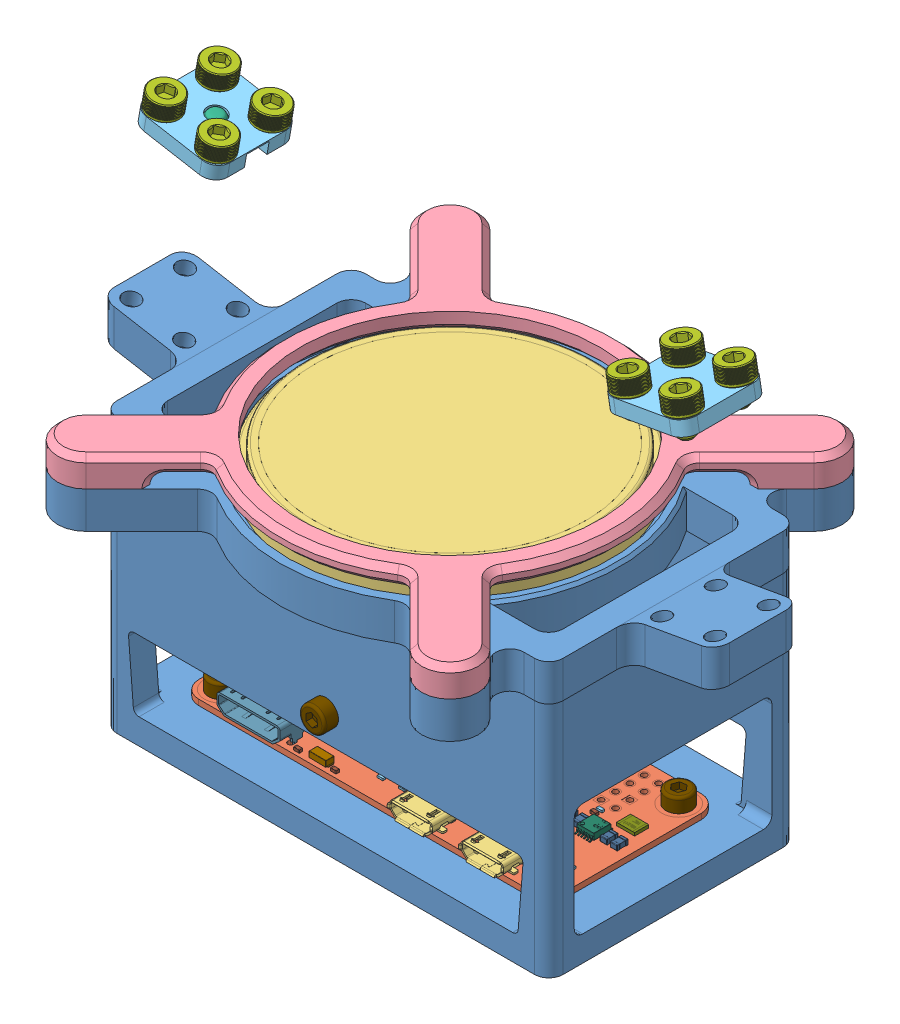
SolidWorks assembly Camera_Case_V1, configuration Default. Lengths in mm.
Overall size (109 86.17 76.19).
152 component instances, 36 part files, 45 mates.
Components (placement in the parent):
- FILTER_MOUNT-1: FILTER_MOUNT [Default] at (13.2312 42.9687 75.706) size (109 9.14 74.46)
- neodymium-1: neodymium [6x3] at (45.4614 49.3687 43.4758) x (0.944555 0 -0.328353) z (-0.328353 0 -0.944555) size (6 3 6)
- neodymium-10: neodymium [3x2] at (50.2312 42.9687 56.206) x (0.999996 0 0.002671) z (-0.002671 0 0.999996) size (3 2 3)
- LENS-1: LENS [Default] at (13.2312 47.4687 75.706) x (-0.754116 0 0.656742) z (-0.656742 0 -0.754116) size (54 5.6 54)
- FILTER_MOUNT_COVER-1: FILTER_MOUNT_COVER [Default] at (13.2312 49.4687 75.706) size (74.46 5 74.46)
- neodymium-2: neodymium [6x3] at (45.4614 49.4687 43.4758) x (-0.92324 0 -0.384223) z (0.384223 0 -0.92324) size (6 3 6)
- neodymium-3: neodymium [6x3] at (45.4614 49.3687 107.9363) x (0.944555 0 0.328353) z (0.328353 0 -0.944555) size (6 3 6)
- neodymium-4: neodymium [6x3] at (45.4614 49.4687 107.9363) x (-0.92324 0 0.384223) z (-0.384223 0 -0.92324) size (6 3 6)
- neodymium-5: neodymium [6x3] at (-18.9991 49.3687 43.4758) x (-0.944555 0 -0.328353) z (-0.328353 0 0.944555) size (6 3 6)
- neodymium-6: neodymium [6x3] at (-18.9991 49.3687 107.9363) x (-0.944555 0 0.328353) z (0.328353 0 0.944555) size (6 3 6)
- neodymium-7: neodymium [6x3] at (-18.9991 49.4687 107.9363) x (0.92324 0 0.384223) z (-0.384223 0 0.92324) size (6 3 6)
- neodymium-8: neodymium [6x3] at (-18.9991 49.4687 43.4758) x (0.92324 0 -0.384223) z (0.384223 0 0.92324) size (6 3 6)
- LED_COVER-1: LED_COVER [Default] at (54.5876 82.7974 75.706) x (0 0 -1) z (-0.984808 -0.173648 0) size (15 2.5 15)
- LED_COVER-2: LED_COVER [Default] at (-28.1253 82.7974 75.706) x (0 0 1) z (0.984808 -0.173648 0) size (15 2.5 15)
- SFH_4716AS_20151008_geometry-1: SFH_4716AS_20151008_geometry [Standard] at (-28.3361 81.6017 75.706) x (-0.984808 0.173648 0) z (0.173648 0.984808 0) size (3.75 3.75 1.55)
- SFH_4716AS_20151008_geometry-2: SFH_4716AS_20151008_geometry [Standard] at (54.7984 81.6017 75.706) x (-0.984808 -0.173648 0) z (-0.173648 0.984808 0) size (3.75 3.75 1.55)
- hex_socket_cylindrical_head_M3.0x4.step-1: hex_socket_cylindrical_head_M3.0x4.step [Default] at (-32.8899 83.1299 80.456) x (-0.968481 0.170769 -0.181335) z (0.173648 0.984808 0) size (5.5 5.5 7.01)
- hex_socket_cylindrical_head_M3.0x4.step-7: hex_socket_cylindrical_head_M3.0x4.step [Default] at (59.3523 83.1299 80.456) x (0.968481 0.170769 -0.181335) z (-0.173648 0.984808 0) size (5.5 5.5 7.01)
- hex_socket_cylindrical_head_M3.0x4.step-3: hex_socket_cylindrical_head_M3.0x4.step [Default] at (-23.5343 81.4802 80.456) x (0.968481 -0.170769 -0.181335) z (0.173648 0.984808 0) size (5.5 5.5 7.01)
- hex_socket_cylindrical_head_M3.0x4.step-8: hex_socket_cylindrical_head_M3.0x4.step [Default] at (49.9966 81.4802 80.456) x (-0.968481 -0.170769 -0.181335) z (-0.173648 0.984808 0) size (5.5 5.5 7.01)
- hex_socket_cylindrical_head_M3.0x4.step-2: hex_socket_cylindrical_head_M3.0x4.step [Default] at (-32.8899 83.1299 70.956) x (-0.968481 0.170769 0.181335) z (0.173648 0.984808 0) size (5.5 5.5 7.01)
- hex_socket_cylindrical_head_M3.0x4.step-6: hex_socket_cylindrical_head_M3.0x4.step [Default] at (59.3523 83.1299 70.956) x (0.968481 0.170769 0.181335) z (-0.173648 0.984808 0) size (5.5 5.5 7.01)
- hex_socket_cylindrical_head_M3.0x4.step-4: hex_socket_cylindrical_head_M3.0x4.step [Default] at (-23.5343 81.4802 70.956) x (0.968481 -0.170769 0.181335) z (0.173648 0.984808 0) size (5.5 5.5 7.01)
- hex_socket_cylindrical_head_M3.0x4.step-5: hex_socket_cylindrical_head_M3.0x4.step [Default] at (49.9966 81.4802 70.956) x (-0.968481 -0.170769 0.181335) z (-0.173648 0.984808 0) size (5.5 5.5 7.01)
- PI_CAM_MOUNT-1: PI_CAM_MOUNT [Default] at (13.2312 20.2317 75.706) x (-1 0 0) z (0 0 -1) size (24.75 5 38)
- M2x1.6mm Hex Nut.step-5: M2x1.6mm Hex Nut.step [Default] at (6.4812 20.3687 86.206) x (-0.866025 0 -0.5) z (0 1 0) size (4.63 4.63 1.6)
- M2x1.6mm Hex Nut.step-13: M2x1.6mm Hex Nut.step [Default] at (19.9812 21.9687 86.206) x (0.866025 0 -0.5) z (0 -1 0) size (4.63 4.63 1.6)
- M2x1.6mm Hex Nut.step-12: M2x1.6mm Hex Nut.step [Default] at (6.4812 21.9687 65.206) x (-0.866025 0 0.5) z (0 -1 0) size (4.63 4.63 1.6)
- M2x1.6mm Hex Nut.step-14: M2x1.6mm Hex Nut.step [Default] at (19.9812 20.3687 65.206) x (0.866025 0 0.5) z (0 1 0) size (4.63 4.63 1.6)
- M2x1.6mm Hex Nut.step-7: M2x1.6mm Hex Nut.step [Default] at (6.4812 21.9687 65.206) x (-0.866025 0 0.5) z (0 -1 0) size (4.63 4.63 1.6) (hidden)
- M2x1.6mm Hex Nut.step-6: M2x1.6mm Hex Nut.step [Default] at (19.9812 21.9687 86.206) x (0.866025 0 -0.5) z (0 -1 0) size (4.63 4.63 1.6) (hidden)
- M2x1.6mm Hex Nut.step-8: M2x1.6mm Hex Nut.step [Default] at (19.9812 20.3687 65.206) x (0.866025 0 0.5) z (0 1 0) size (4.63 4.63 1.6) (hidden)
- Camera Module Assem.STEP-1: Camera Module Assem.STEP [Default] at (-2.8699 5.7203 66.7324) x (0 0 1) z (0 1 0) size (25 24 24.98)
  - 15 Pin Ribbon Block Assem.STEP-1: 15 Pin Ribbon Block Assem.STEP [Default] at (0.7567 20.5462 10.9417) x (1 0 0) z (0 -1 0) size (22 2.5 7)
    - 15 Pin Ribbon Block.STEP-1: 15 Pin Ribbon Block.STEP [Default] at (8.217 10.8197 14.6952) size (20 2.5 6)
    - Ribbon Clamp.STEP-1: Ribbon Clamp.STEP [Default] at (8.217 10.8197 14.6952) size (22 2.5 5)
  - PCB 1.STEP-1: PCB 1.STEP [Default] at (8.9736 12.851 19.5114) size (25 24 2.1)
  - Camera Block.STEP-1: Camera Block.STEP [Default] at (8.9736 15.851 20.5114) size (22 13.5 12.5)
  - Camera end.STEP-1: Camera end.STEP [Default] at (8.9736 15.851 27.3922) x (0.999924 0.012337 0) z (0 0 1) size (14 14 17)
  - Lenz.STEP-1: Lenz.STEP [Default] at (8.9736 15.851 43.8922) size (9 9 0.5)
  - 0603 Resistor.STEP-1: 0603 Resistor.STEP [Default] at (2.3268 23.572 20.4882) size (1.75 0.85 0.59)
  - 0603 Resistor.STEP-2: 0603 Resistor.STEP [Default] at (4.5768 23.572 20.4882) size (1.75 0.85 0.59)
  - 0603 Resistor.STEP-3: 0603 Resistor.STEP [Default] at (15.6203 23.5707 20.4857) size (1.75 0.85 0.59)
  - 0603 Resistor.STEP-4: 0603 Resistor.STEP [Default] at (13.3703 23.5707 20.4857) size (1.75 0.85 0.59)
- hex_socket_cylindrical_head_M2.5x06.step-1: hex_socket_cylindrical_head_M2.5x06.step [Default] at (19.9812 26.3317 86.206) x (0.143858 0 0.989598) z (0 1 0) size (4.5 4.5 8.5)
- hex_socket_cylindrical_head_M2.5x06.step-3: hex_socket_cylindrical_head_M2.5x06.step [Default] at (6.4812 26.3317 86.206) x (-0.143858 0 0.989598) z (0 1 0) size (4.5 4.5 8.5)
- hex_socket_cylindrical_head_M2.5x06.step-2: hex_socket_cylindrical_head_M2.5x06.step [Default] at (19.9812 26.3317 65.206) x (0.143858 0 -0.989598) z (0 1 0) size (4.5 4.5 8.5)
- hex_socket_cylindrical_head_M2.5x06.step-4: hex_socket_cylindrical_head_M2.5x06.step [Default] at (6.4812 26.3317 65.206) x (-0.143858 0 -0.989598) z (0 1 0) size (4.5 4.5 8.5)
- hex_socket_cylindrical_head_M2.5x08.step-1: hex_socket_cylindrical_head_M2.5x08.step [Default] at (13.2312 22.7317 53.706) x (-0.82955 -0.558433 0) z (0 0 -1) size (4.5 4.5 10.5)
- neodymium-11: neodymium [3x2] at (50.2312 42.9687 95.206) x (0.999996 0 -0.002671) z (0.002671 0 0.999996) size (3 2 3)
- neodymium-13: neodymium [3x2] at (-23.7688 42.9687 56.206) x (-0.999996 0 0.002671) z (-0.002671 0 -0.999996) size (3 2 3)
- neodymium-15: neodymium [3x2] at (-23.7688 42.9687 95.206) x (-0.999996 0 -0.002671) z (0.002671 0 -0.999996) size (3 2 3)
- neodymium-9: neodymium [3x2] at (50.2312 40.9687 56.206) x (0.988314 0 0.152432) z (-0.152432 0 0.988314) size (3 2 3)
- neodymium-14: neodymium [3x2] at (-23.7688 40.9687 56.206) x (-0.988314 0 0.152432) z (-0.152432 0 -0.988314) size (3 2 3)
- neodymium-12: neodymium [3x2] at (50.2312 40.9687 95.206) x (0.988314 0 -0.152432) z (0.152432 0 0.988314) size (3 2 3)
- neodymium-16: neodymium [3x2] at (-23.7688 40.9687 95.206) x (-0.988314 0 -0.152432) z (0.152432 0 -0.988314) size (3 2 3)
- PI_CASE-1: PI_CASE [Default] at (13.2312 0.9687 75.706) size (79 42 44)
- M2x1.6mm Hex Nut.step-1: M2x1.6mm Hex Nut.step [Default] at (42.2312 2.9687 64.206) x (-0.866025 0 0.5) z (0 -1 0) size (4.63 4.63 1.6)
- M2x1.6mm Hex Nut.step-10: M2x1.6mm Hex Nut.step [Default] at (-15.7688 1.3687 64.206) x (0.866025 0 0.5) z (0 1 0) size (4.63 4.63 1.6)
- M2x1.6mm Hex Nut.step-9: M2x1.6mm Hex Nut.step [Default] at (42.2312 1.3687 87.206) x (-0.866025 0 -0.5) z (0 1 0) size (4.63 4.63 1.6)
- M2x1.6mm Hex Nut.step-11: M2x1.6mm Hex Nut.step [Default] at (-15.7688 2.9687 87.206) x (0.866025 0 -0.5) z (0 -1 0) size (4.63 4.63 1.6)
- M2x1.6mm Hex Nut.step-4: M2x1.6mm Hex Nut.step [Default] at (-15.7688 1.3687 64.206) x (0.866025 0 0.5) z (0 1 0) size (4.63 4.63 1.6) (hidden)
- M2x1.6mm Hex Nut.step-2: M2x1.6mm Hex Nut.step [Default] at (42.2312 1.3687 87.206) x (-0.866025 0 -0.5) z (0 1 0) size (4.63 4.63 1.6)
- M2x1.6mm Hex Nut.step-3: M2x1.6mm Hex Nut.step [Default] at (-15.7688 2.9687 87.206) x (0.866025 0 -0.5) z (0 -1 0) size (4.63 4.63 1.6) (hidden)
- RPi Zero.stp-1: RPi Zero.stp [Default] at (64.4875 -14.6279 62.6518) size (67.53 4.45 31.23)
  - Raspberry_pizero_PCB.stp-1: Raspberry_pizero_PCB.stp [Default] at (-51.2564 20.0966 13.0542) size (65 1 30)
  - Micro USB_input_female (short)-SMT.stp-1: Micro USB_input_female (short)-SMT.stp [Default] at (-42.3564 22.3216 26.5042) size (7.98 2.94 5.43)
  - Micro USB_input_female (short)-SMT.stp-2: Micro USB_input_female (short)-SMT.stp [Default] at (-29.7564 22.3216 26.5042) size (7.98 2.94 5.43)
  - 0204 - Capacitor.stp-1: 0204 - Capacitor.stp [Default] at (-62.4121 21.3466 11.2398) size (1 0.5 0.6)
  - 0204 - Capacitor.stp-2: 0204 - Capacitor.stp [Default] at (-62.4121 21.3466 12.2528) size (1 0.5 0.6)
  - 0204 - Capacitor.stp-3: 0204 - Capacitor.stp [Default] at (-61.8122 21.3466 13.3136) size (1 0.5 0.6)
  - 0204 - Capacitor.stp-4: 0204 - Capacitor.stp [Default] at (-61.8122 21.3466 14.2646) size (1 0.5 0.6)
  - 0204 - Capacitor.stp-5: 0204 - Capacitor.stp [Default] at (-61.8122 21.3466 15.241) size (1 0.5 0.6)
  - 0204 - Capacitor.stp-6: 0204 - Capacitor.stp [Default] at (-61.8122 21.3466 16.2144) size (1 0.5 0.6)
  - 0204 - Capacitor.stp-7: 0204 - Capacitor.stp [Default] at (-61.8122 21.3466 17.2416) size (1 0.5 0.6)
  - 0204 - Capacitor.stp-8: 0204 - Capacitor.stp [Default] at (-62.5919 21.3466 20.9695) size (1 0.5 0.6)
  - 0204 - Capacitor.stp-9: 0204 - Capacitor.stp [Default] at (-62.5919 21.3466 21.919) size (1 0.5 0.6)
  - 0204 - Capacitor.stp-10: 0204 - Capacitor.stp [Default] at (-60.4584 21.3466 22.3712) x (0 0 1) z (-1 0 0) size (1 0.5 0.6)
  - 0204 - Capacitor.stp-11: 0204 - Capacitor.stp [Default] at (-60.0807 21.3466 22.3712) x (0 0 -1) z (1 0 0) size (1 0.5 0.6)
  - 0204 - Capacitor.stp-12: 0204 - Capacitor.stp [Default] at (-59.0466 21.3466 22.3712) x (0 0 -1) z (1 0 0) size (1 0.5 0.6)
  - 0204 - Capacitor.stp-13: 0204 - Capacitor.stp [Default] at (-52.6496 21.3466 22.316) x (0 0 1) z (-1 0 0) size (1 0.5 0.6)
  - 0204 - Capacitor.stp-14: 0204 - Capacitor.stp [Default] at (-52.25 21.3466 22.316) x (0 0 -1) z (1 0 0) size (1 0.5 0.6)
  - 0204 - Capacitor.stp-15: 0204 - Capacitor.stp [Default] at (-51.2398 21.3466 22.316) x (0 0 -1) z (1 0 0) size (1 0.5 0.6)
  - 0204 - Capacitor.stp-16: 0204 - Capacitor.stp [Default] at (-49.1841 21.3466 22.316) x (0 0 -1) z (1 0 0) size (1 0.5 0.6)
  - 0204 - Capacitor.stp-17: 0204 - Capacitor.stp [Default] at (-48.1448 21.3466 22.316) x (0 0 -1) z (1 0 0) size (1 0.5 0.6)
  - 0204 - Capacitor.stp-18: 0204 - Capacitor.stp [Default] at (-46.475 21.3466 21.113) size (1 0.5 0.6)
  - 0204 - Capacitor.stp-19: 0204 - Capacitor.stp [Default] at (-45.7322 21.3466 20.0663) size (1 0.5 0.6)
  - 0204 - Capacitor.stp-20: 0204 - Capacitor.stp [Default] at (-45.7322 21.3466 19.0675) size (1 0.5 0.6)
  - 0204 - Capacitor.stp-21: 0204 - Capacitor.stp [Default] at (-45.7322 21.3466 18.1249) size (1 0.5 0.6)
  - 0204 - Capacitor.stp-22: 0204 - Capacitor.stp [Default] at (-45.7322 21.3466 17.1095) size (1 0.5 0.6)
  - 0204 - Capacitor.stp-23: 0204 - Capacitor.stp [Default] at (-46.3457 21.3466 16.1412) size (1 0.5 0.6)
  - 0204 - Capacitor.stp-24: 0204 - Capacitor.stp [Default] at (-46.3457 21.3466 15.1229) size (1 0.5 0.6)
  - 0204 - Capacitor.stp-25: 0204 - Capacitor.stp [Default] at (-46.3457 21.3466 14.0197) size (1 0.5 0.6)
  - 0204 - Capacitor.stp-26: 0204 - Capacitor.stp [Default] at (-46.3457 21.3466 12.9589) size (1 0.5 0.6)
  - 0204 - Capacitor.stp-27: 0204 - Capacitor.stp [Default] at (-43.6156 21.3466 13.1418) size (1 0.5 0.6)
  - 0204 - Capacitor.stp-28: 0204 - Capacitor.stp [Default] at (-43.6156 21.3466 10.1424) size (1 0.5 0.6)
  - 0204 - Capacitor.stp-29: 0204 - Capacitor.stp [Default] at (-48.9117 21.3466 7.6917) size (1 0.5 0.6)
  - 0204 - Capacitor.stp-30: 0204 - Capacitor.stp [Default] at (-55.4926 21.3466 7.2526) x (0 0 -1) z (1 0 0) size (1 0.5 0.6)
  - 0204 - Capacitor.stp-31: 0204 - Capacitor.stp [Default] at (-53.7932 21.3466 7.2526) x (0 0 1) z (-1 0 0) size (1 0.5 0.6)
  - 0204 - Capacitor.stp-32: 0204 - Capacitor.stp [Default] at (-59.8477 21.3466 7.2526) x (0 0 1) z (-1 0 0) size (1 0.5 0.6)
  - 0204- Resistor.stp-1: 0204- Resistor.stp [Default] at (-43.6109 21.4522 15.4193) x (-1 0 0) z (0 -1 0) size (0.99 0.51 0.36)
  - 0204- Resistor.stp-2: 0204- Resistor.stp [Default] at (-43.6109 21.4522 14.4127) x (-1 0 0) z (0 -1 0) size (0.99 0.51 0.36)
  - 0204- Resistor.stp-3: 0204- Resistor.stp [Default] at (-43.6109 21.4522 12.4047) x (-1 0 0) z (0 -1 0) size (0.99 0.51 0.36)
  - 0204- Resistor.stp-4: 0204- Resistor.stp [Default] at (-42.6936 21.4522 18.4076) x (-1 0 0) z (0 -1 0) size (0.99 0.51 0.36)
  - 0204- Resistor.stp-5: 0204- Resistor.stp [Default] at (-39.831 21.4522 18.1462) x (0 0 1) z (0 -1 0) size (0.99 0.51 0.36)
  - 0204- Resistor.stp-6: 0204- Resistor.stp [Default] at (-61.8169 21.4522 19.8533) x (-1 0 0) z (0 -1 0) size (0.99 0.51 0.36)
  - 0204- Resistor.stp-7: 0204- Resistor.stp [Default] at (-61.8169 21.4522 18.5178) x (-1 0 0) z (0 -1 0) size (0.99 0.51 0.36)
  - 0204- Resistor.stp-8: 0204- Resistor.stp [Default] at (-79.148 21.4522 17.7279) x (-1 0 0) z (0 -1 0) size (0.99 0.51 0.36)
  - 0204- Resistor.stp-9: 0204- Resistor.stp [Default] at (-56.0985 21.4522 7.2479) x (0 0 -1) z (0 -1 0) size (0.99 0.51 0.36)
  - 0204- Resistor.stp-10: 0204- Resistor.stp [Default] at (-28.0827 21.4522 9.5819) x (-1 0 0) z (0 -1 0) size (0.99 0.51 0.36)
  - 0204- Resistor.stp-11: 0204- Resistor.stp [Default] at (-21.8613 21.4522 20.9026) x (-1 0 0) z (0 -1 0) size (0.99 0.51 0.36)
  - CAP-0306.stp-1: CAP-0306.stp [Default] at (-45.8903 21.4966 8.7634) size (1.6 0.8 0.9)
  - CAP-0306.stp-2: CAP-0306.stp [Default] at (-82.0031 21.4966 19.0464) x (0 0 1) z (-1 0 0) size (1.6 0.8 0.9)
  - Raspberry_pizero_BCM2835 with VC4.stp-1: Raspberry_pizero_BCM2835 with VC4.stp [Default] at (-54.1608 21.5466 15.1238) x (1 0 0) z (0 0 -1) size (12 0.65 12)
  - Crystal 3.4x2.4mm.stp-1: Crystal 3.4x2.4mm.stp [Default] at (-65.3089 21.0966 19.2633) size (3.2 1 2.4)
  - 0204- Resistor.stp-12: 0204- Resistor.stp [Default] at (-68.4329 21.4522 5.4384) x (0 0 1) z (0 -1 0) size (0.99 0.51 0.36)
  - 0204- Resistor.stp-13: 0204- Resistor.stp [Default] at (-69.7255 21.4522 5.4384) x (0 0 1) z (0 -1 0) size (0.99 0.51 0.36)
  - 0204- Resistor.stp-14: 0204- Resistor.stp [Default] at (-65.0626 21.4522 16.5355) x (1 0 0) z (0 -1 0) size (0.99 0.51 0.36)
  - 32,768 Khz Crystal.stp-1: 32,768 Khz Crystal.stp [Default] at (-60.5154 21.1428 26.5473) x (0.999848 -0.017452 0) z (0 0 1) size (3.4 1.03 1.5)
  - 0805- Capacitor.stp-1: 0805- Capacitor.stp [Default] at (-51.9496 21.9966 5.2384) x (1 0 0) z (0 -1 0) size (2 1.26 0.91)
  - 0805- Capacitor.stp-2: 0805- Capacitor.stp [Default] at (-51.9496 21.9966 7.3589) x (1 0 0) z (0 -1 0) size (2 1.26 0.91)
  - 0805- Capacitor.stp-3: 0805- Capacitor.stp [Default] at (-37.009 21.9966 22.5384) x (0 0 -1) z (0 -1 0) size (2 1.26 0.91)
  - 0805- Capacitor.stp-4: 0805- Capacitor.stp [Default] at (-29.8247 21.9966 13.3538) x (0 0 1) z (0 -1 0) size (2 1.26 0.91)
  - 0805- Capacitor.stp-5: 0805- Capacitor.stp [Default] at (-27.9052 21.9966 13.3538) x (0 0 -1) z (0 -1 0) size (2 1.26 0.91)
  - 0805- Capacitor.stp-6: 0805- Capacitor.stp [Default] at (-22.8003 21.9966 13.3538) x (0 0 -1) z (0 -1 0) size (2 1.26 0.91)
  - 0805- Capacitor.stp-7: 0805- Capacitor.stp [Default] at (-20.9924 21.9966 13.3538) x (0 0 -1) z (0 -1 0) size (2 1.26 0.91)
  - 0204- Resistor.stp-15: 0204- Resistor.stp [Default] at (-48.8769 21.4522 23.8207) x (1 0 0) z (0 -1 0) size (0.99 0.51 0.36)
  - 0204- Resistor.stp-16: 0204- Resistor.stp [Default] at (-52.4165 21.4522 24.0419) x (1 0 0) z (0 -1 0) size (0.99 0.51 0.36)
  - 0204 - Capacitor.stp-33: 0204 - Capacitor.stp [Default] at (-47.1199 21.3466 23.926) x (0 0 1) z (-1 0 0) size (1 0.5 0.6)
  - 0204 - Capacitor Brown.stp-1: 0204 - Capacitor Brown.stp [Default] at (-57.5817 21.3466 26.803) size (1 0.5 0.6)
  - 0204 - Capacitor Brown.stp-2: 0204 - Capacitor Brown.stp [Default] at (-64.0312 21.3466 26.8794) size (1 0.5 0.6)
  - 0204 - Capacitor Brown.stp-3: 0204 - Capacitor Brown.stp [Default] at (-46.3457 21.3466 12.214) size (1 0.5 0.6)
  - 0204 - Capacitor Brown.stp-4: 0204 - Capacitor Brown.stp [Default] at (-46.3457 21.3466 11.0963) size (1 0.5 0.6)
  - 0204 - Capacitor Brown.stp-5: 0204 - Capacitor Brown.stp [Default] at (-46.3457 21.3466 10.1566) size (1 0.5 0.6)
  - 0204 - Capacitor Brown.stp-6: 0204 - Capacitor Brown.stp [Default] at (-43.6156 21.3466 11.1151) size (1 0.5 0.6)
  - 0204 - Capacitor Brown.stp-7: 0204 - Capacitor Brown.stp [Default] at (-28.0874 21.3466 10.3236) size (1 0.5 0.6)
  - 0204 - Capacitor Brown.stp-8: 0204 - Capacitor Brown.stp [Default] at (-80.6197 21.3466 20.6997) size (1 0.5 0.6)
  - 0204- Resistor.stp-17: 0204- Resistor.stp [Default] at (-78.9105 21.4522 21.1554) x (1 0 0) z (0 -1 0) size (0.99 0.51 0.36)
  - 6-Pin SOT.stp-1: 6-Pin SOT.stp [Default] at (-79.714 21.0966 19.2138) x (0 0 1) z (0 1 0) size (1.5 1.84 0.95)
  - micro sd molex.stp-1: micro sd molex.stp [Default] at (-74.7768 21.6766 -33.0961) x (0 0 1) z (0 1 0) size (11.95 11.4 1.45)
  - hdmi type C.stp-1: hdmi type C.stp [Default] at (-71.3564 22.9466 28.6542) size (12.9 4.05 7.7)
  - Voltage Regulator 3x3mm 12-Pin.stp-1: Voltage Regulator 3x3mm 12-Pin.stp [Default] at (-23.6842 21.0966 12.6105) x (1 0 0) z (0 1 0) size (3 4.1 1.2)
  - 1210 inductor.stp-1: 1210 inductor.stp [Default] at (-46.4963 21.0916 6.3909) x (0 0 1) z (0 1 0) size (3.25 2.64 0.68)
  - 1210 inductor.stp-2: 1210 inductor.stp [Default] at (-22.7405 21.0916 9.2394) x (1 0 0) z (0 1 0) size (3.25 2.64 0.68)
  - 1210 inductor.stp-3: 1210 inductor.stp [Default] at (-28.2854 21.0916 17.6682) x (1 0 0) z (0 1 0) size (3.25 2.64 0.68)
  - 0204 - Capacitor.stp-34: 0204 - Capacitor.stp [Default] at (-48.9117 21.3466 6.5273) size (1 0.5 0.6)
  - Micro SD Card.stp-1: Micro SD Card.stp [Default] at (-95.3228 21.4466 -12.705) x (0 0 1) z (0 1 0) size (11.01 15 1)
- hex_socket_cylindrical_head_M2.5x05.step-1: hex_socket_cylindrical_head_M2.5x05.step [Default] at (42.2312 6.4687 87.206) x (-0.986552 0 -0.163446) z (0 1 0) size (4.5 4.5 7.5)
- hex_socket_cylindrical_head_M2.5x05.step-3: hex_socket_cylindrical_head_M2.5x05.step [Default] at (-15.7688 6.4687 87.206) x (0.986552 0 -0.163446) z (0 1 0) size (4.5 4.5 7.5)
- hex_socket_cylindrical_head_M2.5x05.step-2: hex_socket_cylindrical_head_M2.5x05.step [Default] at (42.2312 6.4687 64.206) x (-0.986552 0 0.163446) z (0 1 0) size (4.5 4.5 7.5)
- hex_socket_cylindrical_head_M2.5x05.step-4: hex_socket_cylindrical_head_M2.5x05.step [Default] at (-15.7688 6.4687 64.206) x (0.986552 0 0.163446) z (0 1 0) size (4.5 4.5 7.5)
- hex_socket_cylindrical_head_M2.5x08.step-2: hex_socket_cylindrical_head_M2.5x08.step [Default] at (13.2312 22.7317 97.706) x (-0.82955 -0.558433 0) z (0 0 1) size (4.5 4.5 10.5)
Mates (geometry in assembly coordinates):
- Coincident1: coincident anti-aligned: plane of PI_CASE-1 through (16.5015 2.9687 81.3705) normal (-0.5 0 -0.866025); plane of M2x1.6mm Hex Nut.step-1 through (44.2312 2.9687 65.3607) normal (0.5 0 0.866025)
- LimitDistance13: limit distance = 0 mm anti-aligned: plane of PI_CASE-1 through (13.2312 2.9687 75.706) normal (0 -1 0); plane of M2x1.6mm Hex Nut.step-1 through (42.2312 2.9687 64.206) normal (0 1 0)
- Coincident3: coincident anti-aligned: plane of PI_CASE-1 through (24.4608 2.9687 56.2557) normal (0.5 0 -0.866025); plane of M2x1.6mm Hex Nut.step-1 through (42.2312 2.9687 66.5154) normal (-0.5 0 0.866025)
- Concentric1: concentric anti-aligned: cylinder of PI_CASE-1 through (42.2312 0.9687 64.206) axis (0 1 0) radius 1.075; cylinder of RPi Zero.stp-1/Raspberry_pizero_PCB.stp-1 through (42.2312 6.4687 64.206) axis (0 -1 0) radius 1.375
- Concentric2: concentric anti-aligned: cylinder of PI_CASE-1 through (-15.7688 0.9687 87.206) axis (0 1 0) radius 1.075; cylinder of RPi Zero.stp-1/Raspberry_pizero_PCB.stp-1 through (-15.7688 6.4687 87.206) axis (0 -1 0) radius 1.375
- LimitDistance1: limit distance = 0 mm anti-aligned: plane of PI_CASE-1 through (13.2312 5.4687 75.706) normal (0 1 0); plane of RPi Zero.stp-1/Raspberry_pizero_PCB.stp-1 through (-16.2688 5.4687 63.706) normal (0 -1 0)
- Coincident5: coincident anti-aligned: plane of PI_CAM_MOUNT-1 through (5.997 22.2317 88.2359) normal (0.5 0 -0.866025); plane of M2x1.6mm Hex Nut.step-5 through (4.4812 20.3687 87.3607) normal (-0.5 0 0.866025)
- Coincident6: coincident anti-aligned: plane of PI_CAM_MOUNT-1 through (17.0903 22.2317 82.3903) normal (-0.5 0 -0.866025); plane of M2x1.6mm Hex Nut.step-5 through (6.4812 20.3687 88.5154) normal (0.5 0 0.866025)
- LimitDistance15: limit distance = 0.2629 mm anti-aligned: plane of PI_CAM_MOUNT-1 through (13.2312 22.2317 75.706) normal (0 -1 0); plane of M2x1.6mm Hex Nut.step-5 through (6.4812 21.9687 86.206) normal (0 1 0)
- LimitDistance3: limit distance = 0.2629 mm anti-aligned: plane of PI_CASE-1 through (13.2312 19.9687 75.706) normal (0 1 0); plane of PI_CAM_MOUNT-1 through (13.2312 20.2317 75.706) normal (0 -1 0)
- Symmetric3: symmetric aligned: plane of PI_CAM_MOUNT-1 through (13.2312 25.2317 56.706) normal (0 0 -1); plane of PI_CAM_MOUNT-1 through (13.2312 25.2317 94.706) normal (0 0 1)
- Symmetric4: symmetric aligned: plane of PI_CAM_MOUNT-1 through (0.8562 25.2317 75.706) normal (-1 0 0); plane of PI_CAM_MOUNT-1 through (25.6062 25.2317 75.706) normal (1 0 0)
- Concentric5: concentric anti-aligned: cylinder of PI_CAM_MOUNT-1 through (19.9812 25.2317 86.206) axis (0 -1 0) radius 1.075; cylinder of Camera Module Assem.STEP-1/PCB 1.STEP-1 through (19.9812 24.2317 86.206) axis (0 1 0) radius 1
- Concentric6: concentric anti-aligned: cylinder of PI_CAM_MOUNT-1 through (19.9812 25.2317 65.206) axis (0 -1 0) radius 1.075; cylinder of Camera Module Assem.STEP-1/PCB 1.STEP-1 through (19.9812 24.2317 65.206) axis (0 1 0) radius 1
- Coincident15: coincident anti-aligned: plane of PI_CAM_MOUNT-1 through (13.2312 25.2317 75.706) normal (0 1 0); plane of Camera Module Assem.STEP-1/PCB 1.STEP-1 through (9.9812 25.2317 75.706) normal (0 -1 0)
- Concentric7: concentric anti-aligned: cylinder of PI_CASE-1 through (-23.7688 40.5687 56.206) axis (0 1 0) radius 1.625; cylinder of FILTER_MOUNT-1 through (-23.7688 47.4687 56.206) axis (0 -1 0) radius 1.625
- Concentric8: concentric anti-aligned: cylinder of PI_CASE-1 through (50.2312 40.5687 95.206) axis (0 1 0) radius 1.625; cylinder of FILTER_MOUNT-1 through (50.2312 47.4687 95.206) axis (0 -1 0) radius 1.625
- LimitDistance4: limit distance = 0 mm anti-aligned: plane of FILTER_MOUNT-1 through (13.2312 42.9687 75.706) normal (0 -1 0); plane of PI_CASE-1 through (13.2312 42.9687 75.706) normal (0 1 0)
- Concentric9: concentric aligned: cylinder of FILTER_MOUNT-1 through (13.2312 49.4687 75.706) axis (0 -1 0) radius 28.5; cylinder of LENS-1 through (13.2312 51.0687 75.706) axis (0 -1 0) radius 27
- Coincident19: coincident anti-aligned: plane of FILTER_MOUNT-1 through (13.2312 47.4687 75.706) normal (0 1 0); plane of LENS-1 through (13.2312 47.4687 75.706) normal (0 -1 0)
- Concentric10: concentric anti-aligned: circle of FILTER_MOUNT_COVER-1; cylinder of FILTER_MOUNT-1 through (13.2312 47.4687 75.706) axis (0 -1 0) radius 23
- Coincident20: coincident aligned: plane of FILTER_MOUNT-1 through (9.6956 47.4687 79.2416) normal (-0.707107 0 0.707107); plane of FILTER_MOUNT_COVER-1 through (9.6956 54.4687 79.2416) normal (-0.707107 0 0.707107)
- LimitDistance5: limit distance = 0 mm anti-aligned: plane of FILTER_MOUNT-1 through (45.4614 49.4687 43.4758) normal (0 1 0); plane of FILTER_MOUNT_COVER-1 through (13.2312 49.4687 75.706) normal (0 -1 0)
- Concentric11: concentric anti-aligned: circle of FILTER_MOUNT-1; circle of LED_COVER-1
- Concentric12: concentric anti-aligned: circle of FILTER_MOUNT-1; circle of LED_COVER-1
- LimitDistance6: limit distance = 30 mm anti-aligned: plane of LED_COVER-1 through (55.0217 80.3354 75.706) normal (0.173648 -0.984808 0); plane of FILTER_MOUNT-1 through (52.7312 49.4687 68.206) normal (-0.173648 0.984808 0)
- Concentric15: concentric anti-aligned: circle of Camera Module Assem.STEP-1/PCB 1.STEP-1; circle of hex_socket_cylindrical_head_M2.5x06.step-1
- LimitDistance7: limit distance = 0 mm anti-aligned: plane of hex_socket_cylindrical_head_M2.5x06.step-4 through (6.4812 26.3317 65.206) normal (0 -1 0); plane of Camera Module Assem.STEP-1/PCB 1.STEP-1 through (9.9812 26.3317 75.706) normal (0 1 0)
- Concentric16: concentric aligned: circle of RPi Zero.stp-1/Raspberry_pizero_PCB.stp-1; circle of hex_socket_cylindrical_head_M2.5x05.step-1
- LimitDistance8: limit distance = 0 mm anti-aligned: plane of hex_socket_cylindrical_head_M2.5x05.step-1 through (42.2312 6.4687 87.206) normal (0 -1 0); plane of RPi Zero.stp-1/Raspberry_pizero_PCB.stp-1 through (42.2312 6.4687 87.206) normal (0 1 0)
- Concentric17: concentric aligned: circle of LED_COVER-2; circle of SFH_4716AS_20151008_geometry-1
- Parallel1: parallel aligned: line of LED_COVER-2 through (-26.0223 81.7666 73.706) axis (0 0 1); line of SFH_4716AS_20151008_geometry-1 through (-26.3916 81.8317 73.831) axis (0 0 1)
- LimitDistance10: limit distance = 0 mm anti-aligned: plane of SFH_4716AS_20151008_geometry-1 through (-30.0847 82.4829 73.831) normal (0.173648 0.984808 0); plane of LED_COVER-2 through (-28.2381 82.1573 75.706) normal (-0.173648 -0.984808 0)
- Concentric18: concentric aligned: circle of LED_COVER-2; circle of hex_socket_cylindrical_head_M3.0x4.step-1
- LimitDistance11: limit distance = 0 mm anti-aligned: plane of LED_COVER-2 through (-28.1253 82.7974 75.706) normal (0.173648 0.984808 0); plane of hex_socket_cylindrical_head_M3.0x4.step-1 through (-30.2851 83.1783 80.9275) normal (-0.173648 -0.984808 0)
- Concentric19: concentric anti-aligned: circle of FILTER_MOUNT-1; circle of neodymium-1
- LimitDistance16: limit distance = 0 mm anti-aligned: plane of FILTER_MOUNT-1 through (45.4614 46.3687 43.4758) normal (0 1 0); plane of neodymium-1 through (45.4614 46.3687 43.4758) normal (0 -1 0)
- Concentric20: concentric aligned: circle of FILTER_MOUNT_COVER-1; circle of neodymium-2
- LimitDistance18: limit distance = 0 mm aligned: plane of FILTER_MOUNT_COVER-1 through (13.2312 49.4687 75.706) normal (0 -1 0); plane of neodymium-2 through (45.4614 49.4687 43.4758) normal (0 -1 0)
- Concentric21: concentric aligned: circle of PI_CASE-1; circle of neodymium-9
- LimitDistance14: limit distance = 0 mm aligned: plane of PI_CASE-1 through (13.2312 42.9687 75.706) normal (0 1 0); plane of neodymium-9 through (50.2312 42.9687 56.206) normal (0 1 0)
- Concentric22: concentric aligned: circle of FILTER_MOUNT-1; circle of neodymium-10
- LimitDistance17: limit distance = 0 mm aligned: plane of FILTER_MOUNT-1 through (13.2312 42.9687 75.706) normal (0 -1 0); plane of neodymium-10 through (50.2312 42.9687 56.206) normal (0 -1 0)
- Concentric23: concentric anti-aligned: circle of hex_socket_cylindrical_head_M2.5x08.step-1; circle of PI_CAM_MOUNT-1
- LimitDistance12: limit distance = 0 mm anti-aligned: plane of PI_CASE-1 through (13.2312 42.9687 53.706) normal (0 0 -1); plane of hex_socket_cylindrical_head_M2.5x08.step-1 through (13.2312 22.7317 53.706) normal (0 0 1)
